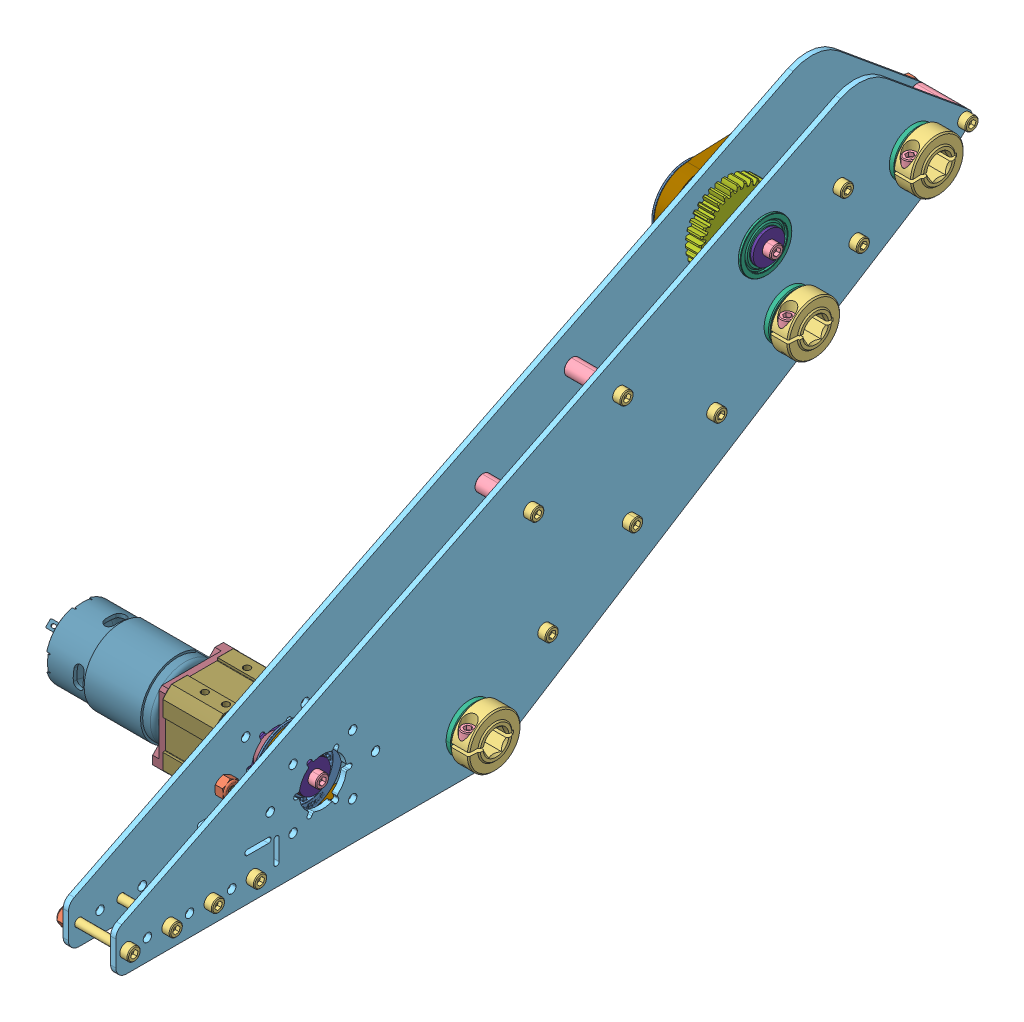
SolidWorks assembly Right_Claw_Assembly, configuration Default. Lengths in mm.
Overall size (171.2 247.71 517.55).
125 component instances, 35 part files, 0 mates.
Components (placement in the parent):
- 9mm wide 24T 500 Hex.STEP-1: 9mm wide 24T 500 Hex.STEP [Default] at (375.9591 173.9174 489.4692) x (1 0 0) z (0 0.018419 0.99983) size (14 42 42)
  - am-3403 24 tooth HTD pulley half 500hex.STEP-1: am-3403 24 tooth HTD pulley half 500hex.STEP [Default] at (-136.5229 43.891 78.8344) size (8.91 42 42)
  - am-3403 24 tooth HTD pulley half 500hex.STEP-2: am-3403 24 tooth HTD pulley half 500hex.STEP [Default] at (-136.5229 43.891 36.8344) x (-1 0 0) z (0 0 -1) size (8.91 42 42)
- 9mm wide 24T 500 Hex.STEP-2: 9mm wide 24T 500 Hex.STEP [Default] at (351.0194 381.3222 230.4036) x (1 0 0) z (0 -0.838389 0.545072) size (14 42 42)
  - am-3403 24 tooth HTD pulley half 500hex.STEP-1: am-3403 24 tooth HTD pulley half 500hex.STEP [Default] at (-136.5229 43.891 78.8344) size (8.91 42 42)
  - am-3403 24 tooth HTD pulley half 500hex.STEP-2: am-3403 24 tooth HTD pulley half 500hex.STEP [Default] at (-136.5229 43.891 36.8344) x (-1 0 0) z (0 0 -1) size (8.91 42 42)
- 9mm wide 24T 500 Hex.STEP-3: 9mm wide 24T 500 Hex.STEP [Default] at (349.4573 384.489 140.1259) x (1 0 0) z (0 -0.834137 0.551557) size (14 42 42)
  - am-3403 24 tooth HTD pulley half 500hex.STEP-1: am-3403 24 tooth HTD pulley half 500hex.STEP [Default] at (-136.5229 43.891 78.8344) size (8.91 42 42)
  - am-3403 24 tooth HTD pulley half 500hex.STEP-2: am-3403 24 tooth HTD pulley half 500hex.STEP [Default] at (-136.5229 43.891 36.8344) x (-1 0 0) z (0 0 -1) size (8.91 42 42)
- 9mm wide 24T 500 Hex.STEP-4: 9mm wide 24T 500 Hex.STEP [Default] at (375.9591 191.0878 396.7517) x (1 0 0) z (0 -0.5 0.866025) size (14 42 42)
  - am-3403 24 tooth HTD pulley half 500hex.STEP-1: am-3403 24 tooth HTD pulley half 500hex.STEP [Default] at (-136.5229 43.891 78.8344) size (8.91 42 42)
  - am-3403 24 tooth HTD pulley half 500hex.STEP-2: am-3403 24 tooth HTD pulley half 500hex.STEP [Default] at (-136.5229 43.891 36.8344) x (-1 0 0) z (0 0 -1) size (8.91 42 42)
- AndyMark Everybot Spacer Subassembly.STEP-1: AndyMark Everybot Spacer Subassembly.STEP [Default] at (54.6794 -110.646 280.1551) size (42.93 11.21 11.21)
  - 10-32 Nylock Nut 1_90631A411.STEP-1: 10-32 Nylock Nut 1_90631A411.STEP [Default] at (168.4198 387.9509 141.8561) x (0 1 0) z (0 0 1) size (9.55 5.96 11.02)
  - 10-32x1500_shcs_HX-SHCS 0.19-32x1.375x1-C.STEP-1: 10-32x1500_shcs_HX-SHCS 0.19-32x1.375x1-C.STEP [Default] at (204.9958 387.9509 141.8561) x (-1 0 0) z (0 -0.673367 0.739309) size (42.93 7.94 7.94)
  - am-3876 1000long .192ID Aluminum Spacer.STEP-1: am-3876 1000long .192ID Aluminum Spacer.STEP [Default] at (171.5948 387.9509 141.8561) x (0 -0.090635 0.995884) z (0 0.995884 0.090635) size (9.53 25.4 9.53)
- AndyMark Everybot Spacer Subassembly.STEP-2: AndyMark Everybot Spacer Subassembly.STEP [Default] at (54.6794 -37.8081 18.3964) size (42.93 11.21 11.21)
  - 10-32 Nylock Nut 1_90631A411.STEP-1: 10-32 Nylock Nut 1_90631A411.STEP [Default] at (168.4198 387.9509 141.8561) x (0 1 0) z (0 0 1) size (9.55 5.96 11.02)
  - 10-32x1500_shcs_HX-SHCS 0.19-32x1.375x1-C.STEP-1: 10-32x1500_shcs_HX-SHCS 0.19-32x1.375x1-C.STEP [Default] at (204.9958 387.9509 141.8561) x (-1 0 0) z (0 -0.673367 0.739309) size (42.93 7.94 7.94)
  - am-3876 1000long .192ID Aluminum Spacer.STEP-1: am-3876 1000long .192ID Aluminum Spacer.STEP [Default] at (171.5948 387.9509 141.8561) x (0 -0.090635 0.995884) z (0 0.995884 0.090635) size (9.53 25.4 9.53)
- AndyMark Everybot Spacer Subassembly.STEP-3: AndyMark Everybot Spacer Subassembly.STEP [Default] at (54.6794 -76.9148 226.3549) size (42.93 11.21 11.21)
  - 10-32 Nylock Nut 1_90631A411.STEP-1: 10-32 Nylock Nut 1_90631A411.STEP [Default] at (168.4198 387.9509 141.8561) x (0 1 0) z (0 0 1) size (9.55 5.96 11.02)
  - 10-32x1500_shcs_HX-SHCS 0.19-32x1.375x1-C.STEP-1: 10-32x1500_shcs_HX-SHCS 0.19-32x1.375x1-C.STEP [Default] at (204.9958 387.9509 141.8561) x (-1 0 0) z (0 -0.673367 0.739309) size (42.93 7.94 7.94)
  - am-3876 1000long .192ID Aluminum Spacer.STEP-1: am-3876 1000long .192ID Aluminum Spacer.STEP [Default] at (171.5948 387.9509 141.8561) x (0 -0.090635 0.995884) z (0 0.995884 0.090635) size (9.53 25.4 9.53)
- AndyMark Everybot Spacer Subassembly.STEP-4: AndyMark Everybot Spacer Subassembly.STEP [Default] at (54.6794 144.8465 -39.0656) x (1 0 0) z (0 -0.832151 0.55455) size (42.93 11.21 11.21)
  - 10-32 Nylock Nut 1_90631A411.STEP-1: 10-32 Nylock Nut 1_90631A411.STEP [Default] at (168.4198 387.9509 141.8561) x (0 1 0) z (0 0 1) size (9.55 5.96 11.02)
  - 10-32x1500_shcs_HX-SHCS 0.19-32x1.375x1-C.STEP-1: 10-32x1500_shcs_HX-SHCS 0.19-32x1.375x1-C.STEP [Default] at (204.9958 387.9509 141.8561) x (-1 0 0) z (0 -0.673367 0.739309) size (42.93 7.94 7.94)
  - am-3876 1000long .192ID Aluminum Spacer.STEP-1: am-3876 1000long .192ID Aluminum Spacer.STEP [Default] at (171.5948 387.9509 141.8561) x (0 -0.090635 0.995884) z (0 0.995884 0.090635) size (9.53 25.4 9.53)
- 57 Sport 4_1 with Flange Mount and 775.STEP-1: 57 Sport 4_1 with Flange Mount and 775.STEP [Default] at (512.1422 191.8089 396.7872) size (148.8 62.86 82.55)
  - am-XXXX - 57 Sport 500 Hex Output Plug.STEP-1: am-XXXX - 57 Sport 500 Hex Output Plug.STEP [Default] at (-295.3931 6.0609 150.085) x (0 0 -1) z (1 0 0) size (44.45 44.45 56.57)
    - am-XXXX - 57 Sport 500 Hex Shaft.STEP-1: am-XXXX - 57 Sport 500 Hex Shaft.STEP [Default] at (0 0 6.1595) x (0.145042 0.989426 0) z (0 0 1) size (14.67 12.71 56.57)
    - Output Block.STEP-1: Output Block.STEP [Default] at origin size (44.45 44.45 20.32)
    - retaining Ring 0500 - Mcm 98410A122_98410A122.STEP-1: retaining Ring 0500 - Mcm 98410A122_98410A122.STEP [Default] at (0 0 -14.5034) x (0 0 1) z (-0.999848 0.017452 0) size (0.89 16.1 14.34)
    - R8ZZ Bearing.STEP-1: R8ZZ Bearing.STEP [Default] at (0 0 6.1595) x (0 0 -1) z (0.975423 0.220339 0) size (7.94 28.57 28.57)
    - R8ZZ Bearing.STEP-2: R8ZZ Bearing.STEP [Default] at (0 0 -5.842) x (0 0 -1) z (0.99707 -0.076493 0) size (7.94 28.57 28.57)
  - am-XXXX - 4_1 Input Stage.STEP-1: am-XXXX - 4_1 Input Stage.STEP [Default] at (-312.8556 6.0609 150.085) x (0 -0.369103 0.929389) z (-1 0 0) size (35.15 35.15 14.63)
    - am-XXXX - 57 Sport Shaft Carrier Plate.STEP-1: am-XXXX - 57 Sport Shaft Carrier Plate.STEP [Default] at origin size (31.12 31.12 14.63)
    - 16T Planet Gear.STEP-1: 16T Planet Gear.STEP [Default] at (-11.8222 1.3023 11.8494) x (0 0 -1) z (1 0 0) size (7.09 12.42 12.42)
    - 16T Planet Gear.STEP-2: 16T Planet Gear.STEP [Default] at (1.3023 11.8222 11.8494) x (0 0 -1) z (0 -1 0) size (7.09 12.42 12.42)
    - 16T Planet Gear.STEP-3: 16T Planet Gear.STEP [Default] at (11.8222 -1.3023 11.8494) x (0 0 -1) z (-1 0 0) size (7.09 12.42 12.42)
    - 16T Planet Gear.STEP-4: 16T Planet Gear.STEP [Default] at (-1.3023 -11.8222 11.8494) x (0 0 -1) z (0 1 0) size (7.09 12.42 12.42)
  - am-4132 57 Sport Flange Mount.STEP-1: am-4132 57 Sport Flange Mount.STEP [Default] at (-295.3931 6.0609 150.085) x (0 0 1) z (0 1 0) size (82.55 6.35 47.62)
  - am-XXXX - 57 Sport 1 Stage Ring Gear Housing.STEP-1: am-XXXX - 57 Sport 1 Stage Ring Gear Housing.STEP [Default] at (-314.3161 6.0609 150.085) x (0 -1 0) z (1 0 0) size (47.63 47.63 31.5)
  - am-3765 - 57 Sport Motor Block.STEP-1: am-3765 - 57 Sport Motor Block.STEP [Default] at (-333.8741 6.0609 150.085) x (0 0 -1) z (1 0 0) size (44.45 44.45 8.89)
  - 775 RedLine.STEP-1: 775 RedLine.STEP [Default] at (-337.6841 6.0609 150.085) x (-1 0 0) z (0 0.707107 -0.707107) size (87.75 44.83 44.07)
  - M4 x .7mm x 8mm SHCS_91290A140.STEP-1: M4 x .7mm x 8mm SHCS_91290A140.STEP [Default] at (-341.9503 -4.1921 139.8319) x (0 -0.977065 0.212941) z (-1 0 0) size (7 7 12.01)
  - M4 Lock Washer_91169A160.STEP-1: M4 Lock Washer_91169A160.STEP [Default] at (-333.1503 -4.1921 139.8319) x (0 0.294925 0.95552) z (-1 0 0) size (7.6 7.6 1.68)
  - M4 x .7mm x 8mm SHCS_91290A140.STEP-2: M4 x .7mm x 8mm SHCS_91290A140.STEP [Default] at (-341.9503 16.314 160.338) x (0 -0.411961 0.911202) z (-1 0 0) size (7 7 12.01)
  - M4 Lock Washer_91169A160.STEP-2: M4 Lock Washer_91169A160.STEP [Default] at (-333.0699 16.314 160.338) x (0 -0.95552 -0.294925) z (1 0 0) size (7.6 7.6 1.68)
  - am-3784 - RS-700 Motor Pinion Gear.STEP-1: am-3784 - RS-700 Motor Pinion Gear.STEP [Default] at (-323.5158 4.9342 148.4301) size (11.94 12.42 12.42)
  - 10-32 x 1.750 SHCS_90128A953.STEP-1: 10-32 x 1.750 SHCS_90128A953.STEP [Default] at (-339.8431 24.0214 132.1245) x (0 0.297258 -0.954797) z (-1 0 0) size (7.92 7.92 49.28)
  - 10-32 x 1.750 SHCS_90128A953.STEP-2: 10-32 x 1.750 SHCS_90128A953.STEP [Default] at (-339.8431 -11.8996 168.0455) x (0 -0.297258 0.954797) z (-1 0 0) size (7.92 7.92 49.28)
  - Thrust washer - 775 Sport.STEP-1: Thrust washer - 775 Sport.STEP [Default] at (-329.01 6.0609 150.085) x (0 0 -1) z (1 0 0) size (31 31 1.52)
  - BHCS 10-32 x 0.500_91255A265.STEP-1: BHCS 10-32 x 0.500_91255A265.STEP [Default] at (-289.6527 24.0214 168.0455) x (0 0 -1) z (1 0 0) size (9.17 9.17 15.27)
  - BHCS 10-32 x 0.500_91255A265.STEP-2: BHCS 10-32 x 0.500_91255A265.STEP [Default] at (-289.6527 -11.8996 132.1245) x (0 0 -1) z (1 0 0) size (9.17 9.17 15.27)
- am-1526 500Hex Collar Clamp.STEP-1: am-1526 500Hex Collar Clamp.STEP [Default] at (238.9418 338.5749 286.0754) x (0 0.052851 0.998602) z (-1 0 0) size (31.72 31.75 12.7)
  - 500Hex Collar Clamp Body.STEP-1: 500Hex Collar Clamp Body.STEP [Default] at (-94.2794 15.3021 33.01) size (31.72 31.75 12.7)
  - 10-32x0500_shcs_HX-SHCS 0.19-32x1.375x1-C.STEP-1: 10-32x0500_shcs_HX-SHCS 0.19-32x1.375x1-C.STEP [Default] at (-83.1669 24.3191 39.36) x (0 -1 0) z (0 0 1) size (17.53 7.94 7.94)
- am-1526 500Hex Collar Clamp.STEP-2: am-1526 500Hex Collar Clamp.STEP [Default] at (303.7214 290.7812 360.5945) x (0 0.052851 0.998602) z (-1 0 0) size (31.72 31.75 12.7)
  - 500Hex Collar Clamp Body.STEP-1: 500Hex Collar Clamp Body.STEP [Default] at (-94.2794 15.3021 33.01) size (31.72 31.75 12.7)
  - 10-32x0500_shcs_HX-SHCS 0.19-32x1.375x1-C.STEP-1: 10-32x0500_shcs_HX-SHCS 0.19-32x1.375x1-C.STEP [Default] at (-83.1669 24.3191 39.36) x (0 -1 0) z (0 0 1) size (17.53 7.94 7.94)
- am-1526 500Hex Collar Clamp.STEP-3: am-1526 500Hex Collar Clamp.STEP [Default] at (303.7214 330.6759 284.8827) x (0 -0.030782 0.999526) z (-1 0 0) size (31.72 31.75 12.7)
  - 500Hex Collar Clamp Body.STEP-1: 500Hex Collar Clamp Body.STEP [Default] at (-94.2794 15.3021 33.01) size (31.72 31.75 12.7)
  - 10-32x0500_shcs_HX-SHCS 0.19-32x1.375x1-C.STEP-1: 10-32x0500_shcs_HX-SHCS 0.19-32x1.375x1-C.STEP [Default] at (-83.1669 24.3191 39.36) x (0 -1 0) z (0 0 1) size (17.53 7.94 7.94)
- am-1526 500Hex Collar Clamp.STEP-4: am-1526 500Hex Collar Clamp.STEP [Default] at (303.7214 171.6969 553.2396) x (0 0.052851 0.998602) z (-1 0 0) size (31.72 31.75 12.7)
  - 500Hex Collar Clamp Body.STEP-1: 500Hex Collar Clamp Body.STEP [Default] at (-94.2794 15.3021 33.01) size (31.72 31.75 12.7)
  - 10-32x0500_shcs_HX-SHCS 0.19-32x1.375x1-C.STEP-1: 10-32x0500_shcs_HX-SHCS 0.19-32x1.375x1-C.STEP [Default] at (-83.1669 24.3191 39.36) x (0 -1 0) z (0 0 1) size (17.53 7.94 7.94)
- AndyMark Everybot Spacer Subassembly.STEP-5: AndyMark Everybot Spacer Subassembly.STEP [Default] at (54.6794 509.1158 698.3459) x (1 0 0) z (0 0.399295 -0.916823) size (42.93 11.21 11.21)
  - 10-32 Nylock Nut 1_90631A411.STEP-1: 10-32 Nylock Nut 1_90631A411.STEP [Default] at (168.4198 387.9509 141.8561) x (0 1 0) z (0 0 1) size (9.55 5.96 11.02)
  - 10-32x1500_shcs_HX-SHCS 0.19-32x1.375x1-C.STEP-1: 10-32x1500_shcs_HX-SHCS 0.19-32x1.375x1-C.STEP [Default] at (204.9958 387.9509 141.8561) x (-1 0 0) z (0 -0.673367 0.739309) size (42.93 7.94 7.94)
  - am-3876 1000long .192ID Aluminum Spacer.STEP-1: am-3876 1000long .192ID Aluminum Spacer.STEP [Default] at (171.5948 387.9509 141.8561) x (0 -0.090635 0.995884) z (0 0.995884 0.090635) size (9.53 25.4 9.53)
- AndyMark Everybot Spacer Subassembly.STEP-6: AndyMark Everybot Spacer Subassembly.STEP [Default] at (54.6794 618.5172 510.7294) x (1 0 0) z (0 0.399295 -0.916823) size (42.93 11.21 11.21)
  - 10-32 Nylock Nut 1_90631A411.STEP-1: 10-32 Nylock Nut 1_90631A411.STEP [Default] at (168.4198 387.9509 141.8561) x (0 1 0) z (0 0 1) size (9.55 5.96 11.02)
  - 10-32x1500_shcs_HX-SHCS 0.19-32x1.375x1-C.STEP-1: 10-32x1500_shcs_HX-SHCS 0.19-32x1.375x1-C.STEP [Default] at (204.9958 387.9509 141.8561) x (-1 0 0) z (0 -0.673367 0.739309) size (42.93 7.94 7.94)
  - am-3876 1000long .192ID Aluminum Spacer.STEP-1: am-3876 1000long .192ID Aluminum Spacer.STEP [Default] at (171.5948 387.9509 141.8561) x (0 -0.090635 0.995884) z (0 0.995884 0.090635) size (9.53 25.4 9.53)
- AndyMark Everybot Spacer Subassembly.STEP-7: AndyMark Everybot Spacer Subassembly.STEP [Default] at (54.6794 572.7943 596.5254) x (1 0 0) z (0 0.399295 -0.916823) size (42.93 11.21 11.21)
  - 10-32 Nylock Nut 1_90631A411.STEP-1: 10-32 Nylock Nut 1_90631A411.STEP [Default] at (168.4198 387.9509 141.8561) x (0 1 0) z (0 0 1) size (9.55 5.96 11.02)
  - 10-32x1500_shcs_HX-SHCS 0.19-32x1.375x1-C.STEP-1: 10-32x1500_shcs_HX-SHCS 0.19-32x1.375x1-C.STEP [Default] at (204.9958 387.9509 141.8561) x (-1 0 0) z (0 -0.673367 0.739309) size (42.93 7.94 7.94)
  - am-3876 1000long .192ID Aluminum Spacer.STEP-1: am-3876 1000long .192ID Aluminum Spacer.STEP [Default] at (171.5948 387.9509 141.8561) x (0 -0.090635 0.995884) z (0 0.995884 0.090635) size (9.53 25.4 9.53)
- AndyMark Everybot Spacer Subassembly.STEP-8: AndyMark Everybot Spacer Subassembly.STEP [Default] at (54.6794 652.0951 520.3355) x (1 0 0) z (0 0.399295 -0.916823) size (42.93 11.21 11.21)
  - 10-32 Nylock Nut 1_90631A411.STEP-1: 10-32 Nylock Nut 1_90631A411.STEP [Default] at (168.4198 387.9509 141.8561) x (0 1 0) z (0 0 1) size (9.55 5.96 11.02)
  - 10-32x1500_shcs_HX-SHCS 0.19-32x1.375x1-C.STEP-1: 10-32x1500_shcs_HX-SHCS 0.19-32x1.375x1-C.STEP [Default] at (204.9958 387.9509 141.8561) x (-1 0 0) z (0 -0.673367 0.739309) size (42.93 7.94 7.94)
  - am-3876 1000long .192ID Aluminum Spacer.STEP-1: am-3876 1000long .192ID Aluminum Spacer.STEP [Default] at (171.5948 387.9509 141.8561) x (0 -0.090635 0.995884) z (0 0.995884 0.090635) size (9.53 25.4 9.53)
- am-4938_in-plate AndyMark EveryBot Intake Plate_V2.STEP-1: am-4938_in-plate AndyMark EveryBot Intake Plate_V2.STEP [Default] at (254.8492 156.5948 671.6871) size (3.17 244.43 516.2)
- am-4938_in-plate AndyMark EveryBot Intake Plate_V2.STEP-2: am-4938_in-plate AndyMark EveryBot Intake Plate_V2.STEP [Default] at (226.2742 156.5948 671.6871) size (3.17 244.43 516.2)
- am-2986 FR8ZZ Hex Bearing.STEP-1: am-2986 FR8ZZ Hex Bearing.STEP [Default] at (256.4494 345.3116 281.1191) x (0 -0.052851 -0.998602) z (0 -0.998602 0.052851) size (31.12 7.94 31.12)
- am-2986 FR8ZZ Hex Bearing.STEP-2: am-2986 FR8ZZ Hex Bearing.STEP [Default] at (221.499 345.3116 281.1191) x (0 0.838389 -0.545072) z (0 0.545072 0.838389) size (31.12 7.94 31.12)
- am-4709 36T 20DP 500hex 375 FW.STEP-1: am-4709 36T 20DP 500hex 375 FW.STEP [Default] at (231.024 345.3116 281.1191) x (1 0 0) z (0 0.891241 0.453531) size (12.7 48.15 48.15)
- am-3948-250 500H x 250IN Spacer.STEP-1: am-3948-250 500H x 250IN Spacer.STEP [Default] at (248.4865 345.3116 281.1191) x (0 0.052851 0.998602) z (-1 0 0) size (20 20 6.35)
- am-4902 60T 5mm HTD Belt 9mm Wide.STEP-1: am-4902 60T 5mm HTD Belt 9mm Wide.STEP [Default] at (208.9344 345.3144 281.0487) x (1 0 0) z (0 -0.039538 0.999218) size (9 41.68 131.68)
- am-4902 60T 5mm HTD Belt 9mm Wide.STEP-2: am-4902 60T 5mm HTD Belt 9mm Wide.STEP [Default] at (235.4362 197.8698 546.8722) x (1 0 0) z (0 0.176389 0.984321) size (9 41.68 131.68)
- am-1692 2 in. Long 0.5 in OD F-F Steel Standoff_92230A135.STEP-1: am-1692 2 in. Long 0.5 in OD F-F Steel Standoff_92230A135.STEP [Default] at (231.0494 345.3116 281.1191) x (0 -0.453531 0.891241) z (1 0 0) size (14.71 14.77 59.16)
- am-3948-063 500H x 063IN Spacer.STEP-1: am-3948-063 500H x 063IN Spacer.STEP [Default] at (206.0278 345.3116 281.1191) x (0 0.891241 0.453531) z (1 0 0) size (20 20 1.59)
- 10-32x0500_shcs_HX-SHCS 0.19-32x1.375x1-C.STEP-1: 10-32x0500_shcs_HX-SHCS 0.19-32x1.375x1-C.STEP [Default] at (199.6143 345.3116 281.1191) x (1 0 0) z (0 0.014609 0.999893) size (17.53 7.94 7.94)
- 10-32 Nylock Nut 1_90631A411.STEP-1: 10-32 Nylock Nut 1_90631A411.STEP [Default] at (226.2742 197.8698 515.1222) x (0 0.902435 0.430825) z (0 0.430825 -0.902435) size (9.55 5.96 11.02)
- 10-32 Nylock Nut 1_90631A411.STEP-2: 10-32 Nylock Nut 1_90631A411.STEP [Default] at (226.2742 197.8698 578.6222) x (0 0.845049 0.534689) z (0 0.534689 -0.845049) size (9.55 5.96 11.02)
- 10-32x750_shcs_90128A945.STEP-1: 10-32x750_shcs_90128A945.STEP [Default] at (235.7992 197.8698 515.1222) x (0 -0.644782 -0.764367) z (1 0 0) size (7.92 7.92 23.88)
- 10-32x750_shcs_90128A945.STEP-2: 10-32x750_shcs_90128A945.STEP [Default] at (235.7992 197.8698 578.6222) x (0 0 -1) z (1 0 0) size (7.92 7.92 23.88)
- am-3948-375 500H x 375IN Spacer.STEP-1: am-3948-375 500H x 375IN Spacer.STEP [Default] at (232.4337 197.8698 546.8722) x (0 0.091272 -0.995826) z (-1 0 0) size (20 20 9.53)
- am-3948-063 500H x 063IN Spacer.STEP-2: am-3948-063 500H x 063IN Spacer.STEP [Default] at (248.0261 197.8698 546.8722) x (0 0.620323 0.784347) z (-1 0 0) size (20 20 1.59)
- am-2986 FR8ZZ Hex Bearing.STEP-3: am-2986 FR8ZZ Hex Bearing.STEP [Default] at (227.8744 348.8728 191.1191) x (0 -0.052851 -0.998602) z (0 -0.998602 0.052851) size (31.12 7.94 31.12)
- am-2986 FR8ZZ Hex Bearing.STEP-4: am-2986 FR8ZZ Hex Bearing.STEP [Default] at (250.074 348.8728 191.1191) x (0 0.902752 0.430162) z (0 -0.430162 0.902752) size (31.12 7.94 31.12)
- am-3948-375 500H x 375IN Spacer.STEP-2: am-3948-375 500H x 375IN Spacer.STEP [Default] at (227.849 348.8728 191.1191) x (0 0.091272 0.995826) z (1 0 0) size (20 20 9.53)
- am-3948-375 500H x 375IN Spacer.STEP-3: am-3948-375 500H x 375IN Spacer.STEP [Default] at (250.0994 301.8828 266.5853) x (0 0.091272 -0.995826) z (-1 0 0) size (20 20 9.53)
- am-4709 36T 20DP 500hex 375 FW.STEP-2: am-4709 36T 20DP 500hex 375 FW.STEP [Default] at (229.4619 301.8828 266.5853) x (1 0 0) z (0 0.813642 0.581366) size (12.7 48.15 48.15)
- am-2986 FR8ZZ Hex Bearing.STEP-5: am-2986 FR8ZZ Hex Bearing.STEP [Default] at (250.074 301.8828 266.5853) x (0 0.902752 0.430162) z (0 -0.430162 0.902752) size (31.12 7.94 31.12)
- am-2986 FR8ZZ Hex Bearing.STEP-6: am-2986 FR8ZZ Hex Bearing.STEP [Default] at (227.8744 301.8828 266.5853) x (0 -0.052851 -0.998602) z (0 -0.998602 0.052851) size (31.12 7.94 31.12)
- am-3948-500 500H x 500IN Spacer.STEP-1: am-3948-500 500H x 500IN Spacer.STEP [Default] at (250.074 348.8728 191.1191) x (0 0 1) z (-1 0 0) size (20 20 12.7)
- am-2986 FR8ZZ Hex Bearing.STEP-7: am-2986 FR8ZZ Hex Bearing.STEP [Default] at (250.074 181.9948 458.2833) x (0 1 0) z (0 0 1) size (31.12 7.94 31.12)
- am-2986 FR8ZZ Hex Bearing.STEP-8: am-2986 FR8ZZ Hex Bearing.STEP [Default] at (227.8744 181.9948 458.2833) x (0 0.381849 -0.924225) z (0 -0.924225 -0.381849) size (31.12 7.94 31.12)
- am-3948-188 500H x 188IN Spacer.STEP-1: am-3948-188 500H x 188IN Spacer.STEP [Default] at (227.8744 181.9948 458.2833) x (0 -0.039215 -0.999231) z (1 0 0) size (20 20 4.78)
- am-3948-125 500H x 125IN Spacer.STEP-1: am-3948-125 500H x 125IN Spacer.STEP [Default] at (246.899 181.9948 458.2833) x (0 -0.062923 0.998018) z (1 0 0) size (20 20 3.17)
- am-1523 10 Fender Washer.STEP-1: am-1523 10 Fender Washer.STEP [Default] at (204.4403 345.3116 281.1191) x (0 -1 0) z (0 0 1) size (19.05 1.59 19.05)
- am-1523 10 Fender Washer.STEP-2: am-1523 10 Fender Washer.STEP [Default] at (256.4494 345.3116 281.1191) x (0 -0.381849 0.924225) z (0 0.924225 0.381849) size (19.05 1.59 19.05)
- 10-32x0500_shcs_HX-SHCS 0.19-32x1.375x1-C.STEP-2: 10-32x0500_shcs_HX-SHCS 0.19-32x1.375x1-C.STEP [Default] at (262.8629 345.3116 281.1191) x (-1 0 0) z (0 -0.924225 -0.381849) size (17.53 7.94 7.94)
- am-1523 10 Fender Washer.STEP-3: am-1523 10 Fender Washer.STEP [Default] at (248.3087 197.8698 546.8722) x (0 -0.381849 0.924225) z (0 0.924225 0.381849) size (19.05 1.59 19.05)
- 10-32x0500_shcs_HX-SHCS 0.19-32x1.375x1-C.STEP-3: 10-32x0500_shcs_HX-SHCS 0.19-32x1.375x1-C.STEP [Default] at (254.7222 197.8698 546.8722) x (-1 0 0) z (0 -0.924225 -0.381849) size (17.53 7.94 7.94)
- 10-32x1500_shcs_HX-SHCS 0.19-32x1.375x1-C.STEP-1: 10-32x1500_shcs_HX-SHCS 0.19-32x1.375x1-C.STEP [Default] at (259.6752 169.2948 589.1371) x (-1 0 0) z (0 -0.673367 0.739309) size (42.93 7.94 7.94)
- 10-32x1500_shcs_HX-SHCS 0.19-32x1.375x1-C.STEP-2: 10-32x1500_shcs_HX-SHCS 0.19-32x1.375x1-C.STEP [Default] at (259.6752 169.2948 614.5371) x (-1 0 0) z (0 -0.673367 0.739309) size (42.93 7.94 7.94)
- 10-32x1500_shcs_HX-SHCS 0.19-32x1.375x1-C.STEP-3: 10-32x1500_shcs_HX-SHCS 0.19-32x1.375x1-C.STEP [Default] at (259.6752 169.2948 639.9371) x (-1 0 0) z (0 -0.673367 0.739309) size (42.93 7.94 7.94)
- 10-32x1500_shcs_HX-SHCS 0.19-32x1.375x1-C.STEP-4: 10-32x1500_shcs_HX-SHCS 0.19-32x1.375x1-C.STEP [Default] at (259.6752 169.2948 665.3371) x (-1 0 0) z (0 -0.673367 0.739309) size (42.93 7.94 7.94)
- 10-32 Nylock Nut 1_90631A411.STEP-3: 10-32 Nylock Nut 1_90631A411.STEP [Default] at (223.0992 169.2948 589.1371) x (0 0.488303 0.872674) z (0 -0.872674 0.488303) size (9.55 5.96 11.02)
- 10-32 Nylock Nut 1_90631A411.STEP-4: 10-32 Nylock Nut 1_90631A411.STEP [Default] at (223.0992 169.2948 614.5371) x (0 0.488303 0.872674) z (0 -0.872674 0.488303) size (9.55 5.96 11.02)
- 10-32 Nylock Nut 1_90631A411.STEP-5: 10-32 Nylock Nut 1_90631A411.STEP [Default] at (223.0992 169.2948 639.9371) x (0 0.488303 0.872674) z (0 -0.872674 0.488303) size (9.55 5.96 11.02)
- 10-32 Nylock Nut 1_90631A411.STEP-6: 10-32 Nylock Nut 1_90631A411.STEP [Default] at (223.0992 169.2948 665.3371) x (0 0.488303 0.872674) z (0 -0.872674 0.488303) size (9.55 5.96 11.02)
